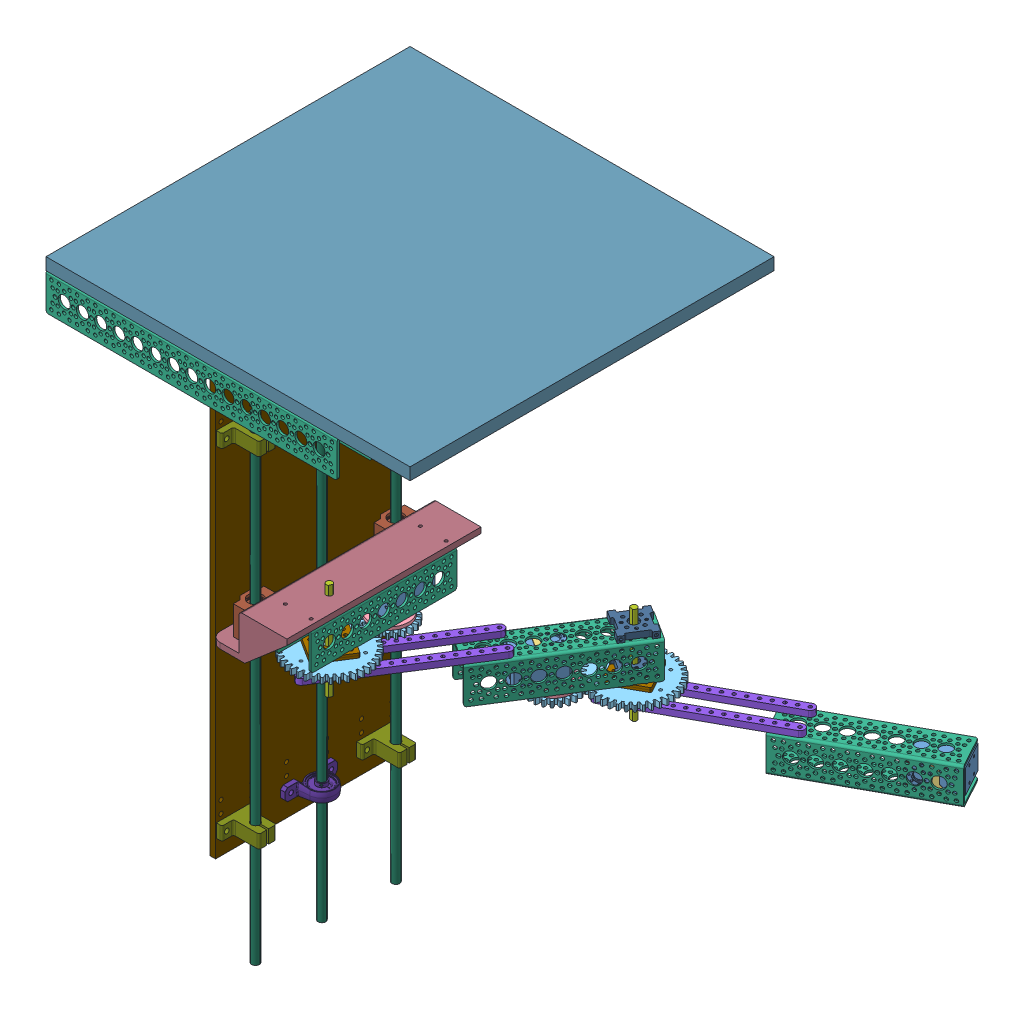
SolidWorks assembly Proto_ASSY, configuration Défaut. Lengths in mm.
Overall size (515.19 647.07 507.57).
91 component instances, 24 part files, 48 mates.
Components (placement in the parent):
- Proto_seg2_ASSY-2: Proto_seg2_ASSY [Défaut] at (38.8897 -351.9425 -94.1656) x (-0.844359 0 -0.535778) z (0 -1 0) size (80 289.98 105.82)
  - XM,H-430_idler-1: XM,H-430_idler [Default] at (3.6223 13.271 44.3) size (28.5 46.5 42.4)
    - XM,H-430_idler.stp-1: XM,H-430_idler.stp [Default] at origin size (28.5 46.5 42.4)
      - X-430_IDLE.stp-1: X-430_IDLE.stp [Default] at origin size (28.5 46.5 42.4)
      - X-430_SPACER_RING.stp-1: X-430_SPACER_RING.stp [Default] at (11 8 14.2) x (-1 0 0) z (0 1 0) size (4.8 2.8 4.8)
      - X-430_SPACER_RING.stp-2: X-430_SPACER_RING.stp [Default] at (-11 8 14.2) x (-1 0 0) z (0 1 0) size (4.8 2.8 4.8)
      - X-430_SPACER_RING.stp-3: X-430_SPACER_RING.stp [Default] at (11 -32 14.2) x (-1 0 0) z (0 1 0) size (4.8 2.8 4.8)
      - X-430_SPACER_RING.stp-4: X-430_SPACER_RING.stp [Default] at (-11 -32 14.2) x (-1 0 0) z (0 1 0) size (4.8 2.8 4.8)
      - X-430_SPACER_RING.stp-5: X-430_SPACER_RING.stp [Default] at (-11 8 -14.2) x (1 0 0) z (0 1 0) size (4.8 2.8 4.8)
      - X-430_SPACER_RING.stp-6: X-430_SPACER_RING.stp [Default] at (11 8 -14.2) x (1 0 0) z (0 1 0) size (4.8 2.8 4.8)
      - X-430_SPACER_RING.stp-7: X-430_SPACER_RING.stp [Default] at (-11 -32 -14.2) x (1 0 0) z (0 1 0) size (4.8 2.8 4.8)
      - X-430_SPACER_RING.stp-8: X-430_SPACER_RING.stp [Default] at (11 -32 -14.2) x (1 0 0) z (0 1 0) size (4.8 2.8 4.8)
      - X-430_CVR_CABLE.stp-1: X-430_CVR_CABLE.stp [Default] at origin size (28.5 12.8 8.8)
  - support_engrenage_proto-1: support_engrenage_proto [Défaut] at (3.6223 13.271 63.3) size (40 40 3.17)
  - Parametric_pinion_V1.1-1: Parametric_pinion_V1.1 [Proto1] at (3.6223 13.271 72.475) x (-0.707107 -0.707107 0) z (0.707107 -0.707107 0) size (47.98 6 47.94)
  - Parametric_pinion_V1.1-2: Parametric_pinion_V1.1 [Proto2] at (1.1079 -157.3492 11.6352) x (-1 0 0) z (0 -1 0) size (80 6 79.96)
  - 585446-1: 585446 [Défaut] at (20.1583 -59.7438 24.3352) x (-1 0 0) z (0 1 0) size (38.1 38.1 152.4)
  - shaft_4po-1: shaft_4po [Défaut] at (1.1083 73.6062 106.8852) x (-0.406647 -0.913585 0) z (0 0 -1) size (5.71 6.35 101.6)
  - 585416-1: 585416 [Défaut] at (14.5787 -103.5672 17.9852) x (0 1 0) z (1 0 0) size (165.99 6.35 9.53)
  - 585416-2: 585416 [Défaut] at (-12.3621 -103.5672 17.9852) x (0 1 0) z (1 0 0) size (165.99 6.35 9.53)
  - 585468-1: 585468 [Défaut] at (1.1079 -157.3492 3.3492) x (0 1 0) z (1 0 0) size (38.1 2.29 38.1)
  - 535130 assembly-1: 535130 assembly [Défaut] at (8.7267 45.2144 39.4652) x (-1 0 0) z (0 1 0) size (33.54 6.36 33.02)
  - 535130 assembly-2: 535130 assembly [Défaut] at (8.7267 45.2144 3.7698) x (-1 0 0) z (0 1 0) size (33.54 6.36 33.02)
  - 535130 assembly-3: 535130 assembly [Défaut] at (-6.5105 -128.9575 -2.5802) x (1 0 0) z (0 -1 0) size (33.54 6.36 33.02)
  - 585468-2: 585468 [Défaut] at (1.1079 -157.3492 1.0632) x (0 1 0) z (1 0 0) size (38.1 2.29 38.1)
- Proto_seg3_ASSY-1: Proto_seg3_ASSY [Défaut] at (314.3259 -437.1175 -265.1335) x (-0.480885 0 -0.876784) z (0.876784 0 -0.480885) size (80 61.37 300.1)
  - 585446-1: 585446 [Défaut] at (0 0 -152.4) x (0 -1 0) z (0 0 1) size (38.1 38.1 152.4)
  - 585416-1: 585416 [Défaut] at (5.5796 0 -206.0024) x (0 0 -1) z (1 0 0) size (165.99 6.35 9.53)
  - 585416-2: 585416 [Défaut] at (32.5204 0 -206.0024) x (0 0 -1) z (1 0 0) size (165.99 6.35 9.53)
  - Parametric_pinion_V1.1-1: Parametric_pinion_V1.1 [Proto2] at (19.0496 12.7 -259.7844) size (80 6 79.96)
  - XM,H-430_idler-1: XM,H-430_idler [Default] at (19.9648 -16.536 -34.9148) x (0 -1 0) z (1 0 0) size (28.5 46.5 42.4)
    - XM,H-430_idler.stp-1: XM,H-430_idler.stp [Default] at origin size (28.5 46.5 42.4)
      - X-430_IDLE.stp-1: X-430_IDLE.stp [Default] at origin size (28.5 46.5 42.4)
      - X-430_SPACER_RING.stp-1: X-430_SPACER_RING.stp [Default] at (11 8 14.2) x (-1 0 0) z (0 1 0) size (4.8 2.8 4.8)
      - X-430_SPACER_RING.stp-2: X-430_SPACER_RING.stp [Default] at (-11 8 14.2) x (-1 0 0) z (0 1 0) size (4.8 2.8 4.8)
      - X-430_SPACER_RING.stp-3: X-430_SPACER_RING.stp [Default] at (11 -32 14.2) x (-1 0 0) z (0 1 0) size (4.8 2.8 4.8)
      - X-430_SPACER_RING.stp-4: X-430_SPACER_RING.stp [Default] at (-11 -32 14.2) x (-1 0 0) z (0 1 0) size (4.8 2.8 4.8)
      - X-430_SPACER_RING.stp-5: X-430_SPACER_RING.stp [Default] at (-11 8 -14.2) x (1 0 0) z (0 1 0) size (4.8 2.8 4.8)
      - X-430_SPACER_RING.stp-6: X-430_SPACER_RING.stp [Default] at (11 8 -14.2) x (1 0 0) z (0 1 0) size (4.8 2.8 4.8)
      - X-430_SPACER_RING.stp-7: X-430_SPACER_RING.stp [Default] at (-11 -32 -14.2) x (1 0 0) z (0 1 0) size (4.8 2.8 4.8)
      - X-430_SPACER_RING.stp-8: X-430_SPACER_RING.stp [Default] at (11 -32 -14.2) x (1 0 0) z (0 1 0) size (4.8 2.8 4.8)
      - X-430_CVR_CABLE.stp-1: X-430_CVR_CABLE.stp [Default] at origin size (28.5 12.8 8.8)
  - 535130 assembly-1: 535130 assembly [Défaut] at (11.4312 -7.8654 -288.1761) size (33.54 6.36 33.02)
  - 585468-1: 585468 [Défaut] at (19.0496 18.7 -259.7844) size (38.1 2.29 38.1)
  - 585468-2: 585468 [Défaut] at (19.0496 20.986 -259.7844) size (38.1 2.29 38.1)
- Proto_seg1_ASSY-1: Proto_seg1_ASSY [Défaut] at (-47.4583 -291.1027 -35.5062) x (1 0 0) z (0 -1 0) size (97.38 203.2 101.6)
  - XM,H-430_idler-1: XM,H-430_idler [Default] at (3.6223 13.271 44.3) size (28.5 46.5 42.4)
    - XM,H-430_idler.stp-1: XM,H-430_idler.stp [Default] at origin size (28.5 46.5 42.4)
      - X-430_IDLE.stp-1: X-430_IDLE.stp [Default] at origin size (28.5 46.5 42.4)
      - X-430_SPACER_RING.stp-1: X-430_SPACER_RING.stp [Default] at (11 8 14.2) x (-1 0 0) z (0 1 0) size (4.8 2.8 4.8)
      - X-430_SPACER_RING.stp-2: X-430_SPACER_RING.stp [Default] at (-11 8 14.2) x (-1 0 0) z (0 1 0) size (4.8 2.8 4.8)
      - X-430_SPACER_RING.stp-3: X-430_SPACER_RING.stp [Default] at (11 -32 14.2) x (-1 0 0) z (0 1 0) size (4.8 2.8 4.8)
      - X-430_SPACER_RING.stp-4: X-430_SPACER_RING.stp [Default] at (-11 -32 14.2) x (-1 0 0) z (0 1 0) size (4.8 2.8 4.8)
      - X-430_SPACER_RING.stp-5: X-430_SPACER_RING.stp [Default] at (-11 8 -14.2) x (1 0 0) z (0 1 0) size (4.8 2.8 4.8)
      - X-430_SPACER_RING.stp-6: X-430_SPACER_RING.stp [Default] at (11 8 -14.2) x (1 0 0) z (0 1 0) size (4.8 2.8 4.8)
      - X-430_SPACER_RING.stp-7: X-430_SPACER_RING.stp [Default] at (-11 -32 -14.2) x (1 0 0) z (0 1 0) size (4.8 2.8 4.8)
      - X-430_SPACER_RING.stp-8: X-430_SPACER_RING.stp [Default] at (11 -32 -14.2) x (1 0 0) z (0 1 0) size (4.8 2.8 4.8)
      - X-430_CVR_CABLE.stp-1: X-430_CVR_CABLE.stp [Default] at origin size (28.5 12.8 8.8)
  - support_engrenage_proto-1: support_engrenage_proto [Défaut] at (3.6223 13.271 63.3) size (40 40 3.17)
  - Parametric_pinion_V1.1-1: Parametric_pinion_V1.1 [Proto1] at (3.6223 13.271 72.475) x (-0.707107 -0.707107 0) z (0.707107 -0.707107 0) size (47.98 6 47.94)
  - 585446-1: 585446 [Défaut] at (-17.9417 111.7062 24.3352) x (1 0 0) z (0 -1 0) size (38.1 38.1 152.4)
  - shaft_4po-1: shaft_4po [Défaut] at (1.1083 73.6062 8.8102) x (0.937211 0.348763 0) z (0 0 1) size (5.71 6.35 101.6)
  - SC8UU 8x34mm Slide Bushing-1: SC8UU 8x34mm Slide Bushing [Default] at (-42.3417 -38.0938 41.3352) x (0 1 0) z (0 0 1) size (34 22 30)
  - SC8UU 8x34mm Slide Bushing-2: SC8UU 8x34mm Slide Bushing [Default] at (-42.3417 109.1062 41.3352) x (0 1 0) z (0 0 1) size (34 22 30)
  - Trapezoidal lead screw Nut tr8x8-4-1: Trapezoidal lead screw Nut tr8x8-4 [Default] at (-44.8417 35.5062 56.3352) x (0 -1 0) z (0 0 1) size (22 22 16.4)
  - proto_bracket_vertical-1: proto_bracket_vertical [Défaut] at (-29.8417 35.5062 40.3352) x (0 1 0) z (1 0 0) size (203.2 44 80)
- base_proto-1: base_proto [Défaut] x (1 0 0) z (0 -1 0) size (381 381 12.7)
- Roto_vertical_sys_ASSY-1: Roto_vertical_sys_ASSY [Défaut] at (-92.3 -282.575 0) x (1 0 0) z (0 0 -1) size (46.88 634.37 190.5)
  - Leadscrew-1: Leadscrew [Défaut] at (4 -135.5 -73.49) x (-0.985183 0 -0.171505) z (0 1 0) size (8 8 500)
  - Leadscrew-2: Leadscrew [Défaut] at (0 -135.5 0) x (-1 0 0) z (0 1 0) size (8 8 500)
  - Leadscrew-3: Leadscrew [Défaut] at (4 -135.5 73.49) x (-0.950264 0 -0.311446) z (0 1 0) size (8 8 500)
  - Linear Rail Shaft Guide-Support - 8mm Diameter - SK8-1: Linear Rail Shaft Guide-Support - 8mm Diameter - SK8 [Default] at (-16 251.475 73.49) x (0 0 -1) z (0 -1 0) size (42 32.8 14)
  - KP08 bearing bracket-1: KP08 bearing bracket [Default] at (-16 244.475 4.0618) x (0 0 -1) z (0 -1 0) size (55 40.88 13.92)
  - KP08 bearing bracket-2: KP08 bearing bracket [Default] at (-16 -111.125 4.0618) x (0 0 -1) z (0 -1 0) size (55 40.88 13.92)
  - Linear Rail Shaft Guide-Support - 8mm Diameter - SK8-2: Linear Rail Shaft Guide-Support - 8mm Diameter - SK8 [Default] at (-16 -104.125 -73.49) x (0 0 -1) z (0 -1 0) size (42 32.8 14)
  - Linear Rail Shaft Guide-Support - 8mm Diameter - SK8-3: Linear Rail Shaft Guide-Support - 8mm Diameter - SK8 [Default] at (-16 251.475 -73.49) x (0 0 -1) z (0 -1 0) size (42 32.8 14)
  - Linear Rail Shaft Guide-Support - 8mm Diameter - SK8-4: Linear Rail Shaft Guide-Support - 8mm Diameter - SK8 [Default] at (-16 -104.125 73.49) x (0 0 -1) z (0 -1 0) size (42 32.8 14)
  - proto_base_verticale-1: proto_base_verticale [Défaut] at (-16 0 0) x (0 0 1) z (-1 0 0) size (190.5 539.75 6)
  - adaptateur-1: adaptateur [Défaut] at (0 -169.35 0) x (0 1 0) z (-1 0 0) size (31.75 12.7 12.7)
  - Cytron 430RPM-1: Cytron 430RPM [Default] at (0 -153.475 0) x (0 -1 0) z (1 0 0) size (113.9 32 32)
  - jaw shaft coupler 5x8mm-1: jaw shaft coupler 5x8mm [Default] at (-55.6153 158.4503 -193.7293) x (0.702573 0 -0.711612) z (0 -1 0) size (20.28 20.28 25.6)
  - proto_motor_bracket-1: proto_motor_bracket [Défaut] at (0 -216.775 0) x (0 0 1) z (0 1 0) size (51 34.5 71)
- 585424-1: 585424 [Défaut] at (-108.3 -31.75 -76.2) x (0 0 1) z (0 1 0) size (38.1 38.1 38.1)
- 585424-2: 585424 [Défaut] at (-108.3 -31.75 76.2) x (0 0 1) z (0 1 0) size (38.1 38.1 38.1)
- 585454-2: 585454 [Défaut] at (-114.3 -12.7 -152.4) x (-1 0 0) z (0 0 1) size (38.1 38.1 304.8)
- 585454-3: 585454 [Défaut] at (114.3 -12.7 190.5) x (0 0 -1) z (-1 0 0) size (38.1 38.1 304.8)
- 585454-4: 585454 [Défaut] at (114.3 -12.7 -152.4) x (0 0 -1) z (-1 0 0) size (38.1 38.1 304.8)
- 585424-3: 585424 [Défaut] at (-152.4 -31.75 -133.35) x (0 -1 0) z (0 0 -1) size (38.1 38.1 38.1)
- 585424-4: 585424 [Défaut] at (-152.4 -31.75 133.35) x (0 1 0) z (0 0 1) size (38.1 38.1 38.1)
- 585424-5: 585424 [Défaut] at (-114.3 -31.75 -133.35) x (0 1 0) z (0 0 -1) size (38.1 38.1 38.1)
- 585424-6: 585424 [Défaut] at (-114.3 -31.75 133.35) x (0 -1 0) z (0 0 1) size (38.1 38.1 38.1)
Mates (geometry in assembly coordinates):
- Coaxiale5: concentric anti-aligned: cylinder of moteur_ass_proto-2/Parametric_pinion_V1.1-2 through (-46.35 -357.5777 38.1) axis (0 -1 0) radius 3.205; cylinder of Proto_seg1_ASSY-1/shaft_4po-1 through (-46.35 -401.5129 38.1) axis (0 1 0) radius 3.175
- Coïncidente14: coincident anti-aligned: plane of base_proto-1 through (0 0 0) normal (0 -1 0)
- Coïncidente15: coincident aligned: plane of base_proto-1 through (0 0 0) normal (0 0 1)
- Coïncidente16: coincident aligned: plane of base_proto-1 through (0 0 0) normal (1 0 0)
- Parallèle2: parallel anti-aligned: plane of Proto_seg1_ASSY-1/585446-1 through (-27.3 -315.4379 -76.2) normal (0 1 0); plane of base_proto-1 through (0 -12.7 0) normal (0 -1 0)
- Parallèle3: parallel aligned: plane of Proto_seg1_ASSY-1/585446-1 through (-65.4 -315.4379 -76.2) normal (0 0 -1); plane of base_proto-1 through (-190.5 -12.7 -190.5) normal (0 0 -1)
- Coïncidente17: coincident anti-aligned: plane of base_proto-1 through (0 -12.7 0) normal (0 -1 0); plane of Roto_vertical_sys_ASSY-1/585454-1 through (-166.7 -12.7 -152.4) normal (0 1 0)
- Largeur1: width anti-aligned: plane of Roto_vertical_sys_ASSY-1/585454-1 through (-204.8 -12.7 152.4) normal (0 0 1); plane of base_proto-1 through (-204.8 -12.7 -152.4) normal (0 0 -1); plane of Roto_vertical_sys_ASSY-1/585454-1 through (-190.5 -12.7 190.5) normal (0 0 1); plane of base_proto-1 through (-190.5 -12.7 -190.5) normal (0 0 -1)
- Distance3: distance = 100 mm aligned: plane of Roto_vertical_sys_ASSY-1/585454-1 through (-204.8 -12.7 -152.4) normal (-1 0 0); plane of base_proto-1 through (-190.5 -12.7 -190.5) normal (-1 0 0)
- Distance5: distance = 76.2 mm aligned: plane of Roto_vertical_sys_ASSY-1/proto_bracket_bearing-2 through (-228.6 -115.3 0) normal (-1 0 0); plane of base_proto-1 through (-190.5 -12.7 -190.5) normal (-1 0 0)
- Largeur2: width anti-aligned: plane of base_proto-1 through (-190.5 -12.7 -190.5) normal (0 0 -1); plane of base_proto-1 through (-190.5 -12.7 190.5) normal (0 0 1); plane of Roto_vertical_sys_ASSY-1/proto_bracket_bearing-2 through (-228.6 -102.6 101.6) normal (0 0 1); plane of Roto_vertical_sys_ASSY-1/proto_bracket_bearing-2 through (-228.6 -102.6 -101.6) normal (0 0 -1)
- Coïncidente20: coincident anti-aligned: plane of Proto_seg1_ASSY-1/585446-1 through (-27.3 -315.4379 -76.2) normal (0 1 0); plane of Roto_vertical_sys_ASSY-1/proto_bracket_vertical-1 through (-191.6 -262.5843 0) normal (0 -1 0)
- Coïncidente21: coincident aligned: plane of Proto_seg1_ASSY-1/585446-1 through (-27.3 -353.5379 -76.2) normal (1 0 0); plane of Roto_vertical_sys_ASSY-1/proto_bracket_vertical-1 through (-131.6 -252.5843 101.6) normal (1 0 0)
- Coaxiale6: concentric anti-aligned: cylinder of Proto_seg1_ASSY-1/proto_bracket_vertical-1 through (-92.3 -315.4379 0) axis (0 -1 0) radius 4.5; cylinder of Roto_vertical_sys_ASSY-1/Leadscrew-2 through (-92.3 -647.075 0) axis (0 1 0) radius 4
- Parallèle4: parallel aligned: plane of Proto_seg1_ASSY-1/proto_bracket_vertical-1 through (-71.3 -331.4379 0) normal (1 0 0); plane of Roto_vertical_sys_ASSY-1/proto_base_verticale-1 through (-108.3 -282.575 0) normal (1 0 0)
- Distance7: distance = 76.2 mm aligned: plane of Roto_vertical_sys_ASSY-1/proto_base_verticale-1 through (-114.3 -282.575 0) normal (-1 0 0); plane of base_proto-1 through (-190.5 -12.7 -190.5) normal (-1 0 0)
- Largeur3: width anti-aligned: plane of base_proto-1 through (-190.5 -12.7 -190.5) normal (0 0 -1); plane of Roto_vertical_sys_ASSY-1/proto_base_verticale-1 through (-190.5 -12.7 190.5) normal (0 0 1); plane of base_proto-1 through (-114.3 -12.7 95.25) normal (0 0 1); plane of Roto_vertical_sys_ASSY-1/proto_base_verticale-1 through (-114.3 -12.7 -95.25) normal (0 0 -1)
- Coïncidente27: coincident anti-aligned: plane of base_proto-1 through (0 -12.7 0) normal (0 -1 0); plane of Roto_vertical_sys_ASSY-1/proto_base_verticale-1 through (-114.3 -12.7 95.25) normal (0 1 0)
- Coïncidente32: coincident anti-aligned: plane of Roto_vertical_sys_ASSY-1/proto_base_verticale-1 through (-108.3 -282.575 0) normal (1 0 0); plane of 585424-1 through (-108.3 -31.75 -76.2) normal (-1 0 0)
- Coïncidente33: coincident anti-aligned: plane of base_proto-1 through (0 -12.7 0) normal (0 -1 0); plane of 585424-1 through (-106.014 -12.7 -95.25) normal (0 1 0)
- Coïncidente34: coincident aligned: plane of Roto_vertical_sys_ASSY-1/proto_base_verticale-1 through (-114.3 -12.7 -95.25) normal (0 0 -1); plane of 585424-1 through (-106.014 -12.7 -95.25) normal (0 0 -1)
- Coïncidente35: coincident anti-aligned: plane of Roto_vertical_sys_ASSY-1/proto_base_verticale-1 through (-108.3 -282.575 0) normal (1 0 0); plane of 585424-2 through (-108.3 -31.75 76.2) normal (-1 0 0)
- Coïncidente36: coincident anti-aligned: plane of base_proto-1 through (0 -12.7 0) normal (0 -1 0); plane of 585424-2 through (-106.014 -12.7 57.15) normal (0 1 0)
- Coïncidente37: coincident aligned: plane of Roto_vertical_sys_ASSY-1/proto_base_verticale-1 through (-114.3 -12.7 95.25) normal (0 0 1); plane of 585424-2 through (-106.014 -12.7 95.25) normal (0 0 1)
- Coïncidente44: coincident anti-aligned: plane of base_proto-1 through (0 -12.7 0) normal (0 -1 0); plane of 585454-2 through (-152.4 -12.7 152.4) normal (0 1 0)
- Coïncidente45: coincident anti-aligned: plane of Roto_vertical_sys_ASSY-1/proto_base_verticale-1 through (-114.3 -282.575 0) normal (-1 0 0); plane of 585454-2 through (-114.3 -12.7 152.4) normal (1 0 0)
- Largeur5: width anti-aligned: plane of 585454-2 through (-114.3 -12.7 152.4) normal (0 0 1); plane of Roto_vertical_sys_ASSY-1/proto_base_verticale-1 through (-114.3 -12.7 -152.4) normal (0 0 -1); plane of 585454-2 through (-114.3 -12.7 -95.25) normal (0 0 -1); plane of Roto_vertical_sys_ASSY-1/proto_base_verticale-1 through (-114.3 -12.7 95.25) normal (0 0 1)
- Coïncidente49: coincident anti-aligned: plane of base_proto-1 through (0 -12.7 0) normal (0 -1 0); plane of 585454-3 through (-190.5 -12.7 152.4) normal (0 1 0)
- Coïncidente51: coincident anti-aligned: plane of base_proto-1 through (0 -12.7 0) normal (0 -1 0); plane of 585454-4 through (-190.5 -12.7 -190.5) normal (0 1 0)
- Coïncidente52: coincident anti-aligned: plane of 585454-2 through (-114.3 -12.7 -152.4) normal (0 0 -1); plane of 585454-4 through (-190.5 -12.7 -152.4) normal (0 0 1)
- Coïncidente53: coincident aligned: plane of 585454-3 through (-190.5 -12.7 190.5) normal (-1 0 0); plane of 585454-4 through (-190.5 -12.7 -152.4) normal (-1 0 0)
- Coïncidente57: coincident aligned: plane of moteur_ass_proto-2/Parametric_pinion_V1.1-1 through (42.9415 -424.4175 -107.3118) normal (0 -1 0); plane of Proto_seg3_ASSY-1/Parametric_pinion_V1.1-1 through (77.3905 -424.4175 -156.9094) normal (0 -1 0)
- Coïncidente60: coincident aligned: plane of moteur_ass_proto-2/Parametric_pinion_V1.1-2 through (-46.35 -363.5777 38.1) normal (0 -1 0); plane of Proto_seg1_ASSY-1/Parametric_pinion_V1.1-1 through (-43.836 -363.5777 -22.2352) normal (0 -1 0)
- Coaxiale8: concentric aligned: cylinder of moteur_ass_proto-2/shaft_4po-1 through (77.3905 -357.2277 -156.9094) axis (0 -1 0) radius 3.175; cylinder of Proto_seg3_ASSY-1/Parametric_pinion_V1.1-1 through (77.3905 -418.4175 -156.9094) axis (0 -1 0) radius 3.205
- Coïncidente61: coincident anti-aligned: plane of 585454-2 through (-152.4 -50.8 152.4) normal (-1 0 0); plane of 585424-3 through (-152.4 -31.75 -133.35) normal (1 0 0)
- Coïncidente62: coincident anti-aligned: plane of 585454-4 through (-190.5 -12.7 -152.4) normal (0 0 1); plane of 585424-3 through (-154.686 -12.7 -152.4) normal (0 0 -1)
- Coïncidente63: coincident anti-aligned: plane of base_proto-1 through (0 -12.7 0) normal (0 -1 0); plane of 585424-3 through (-154.686 -12.7 -152.4) normal (0 1 0)
- Coïncidente64: coincident anti-aligned: plane of 585454-3 through (-190.5 -50.8 152.4) normal (0 0 -1); plane of 585424-4 through (-154.686 -50.8 152.4) normal (0 0 1)
- Coïncidente65: coincident aligned: plane of 585454-4 through (-190.5 -12.7 -152.4) normal (-1 0 0); plane of 585424-3 through (-190.5 -12.7 -150.114) normal (-1 0 0)
- Coïncidente66: coincident anti-aligned: plane of 585454-2 through (-152.4 -50.8 152.4) normal (-1 0 0); plane of 585424-4 through (-152.4 -31.75 133.35) normal (1 0 0)
- Coïncidente67: coincident anti-aligned: plane of base_proto-1 through (0 -12.7 0) normal (0 -1 0); plane of 585424-4 through (-154.686 -12.7 152.4) normal (0 1 0)
- Coïncidente68: coincident anti-aligned: plane of 585454-2 through (-114.3 -12.7 152.4) normal (0 0 1); plane of 585454-3 through (-190.5 -50.8 152.4) normal (0 0 -1)
- Coïncidente69: coincident anti-aligned: plane of 585454-2 through (-114.3 -12.7 152.4) normal (1 0 0); plane of 585424-5 through (-114.3 -31.75 -133.35) normal (-1 0 0)
- Coïncidente70: coincident anti-aligned: plane of 585454-4 through (-190.5 -12.7 -152.4) normal (0 0 1); plane of 585424-5 through (-112.014 -50.8 -152.4) normal (0 0 -1)
- Coïncidente71: coincident anti-aligned: plane of base_proto-1 through (0 -12.7 0) normal (0 -1 0); plane of 585424-5 through (-112.014 -12.7 -152.4) normal (0 1 0)
- Coïncidente72: coincident anti-aligned: plane of 585454-2 through (-114.3 -12.7 152.4) normal (1 0 0); plane of 585424-6 through (-114.3 -31.75 133.35) normal (-1 0 0)
- Coïncidente73: coincident anti-aligned: plane of 585454-3 through (-190.5 -50.8 152.4) normal (0 0 -1); plane of 585424-6 through (-112.014 -12.7 152.4) normal (0 0 1)
- Coïncidente74: coincident anti-aligned: plane of base_proto-1 through (0 -12.7 0) normal (0 -1 0); plane of 585424-6 through (-112.014 -12.7 152.4) normal (0 1 0)
